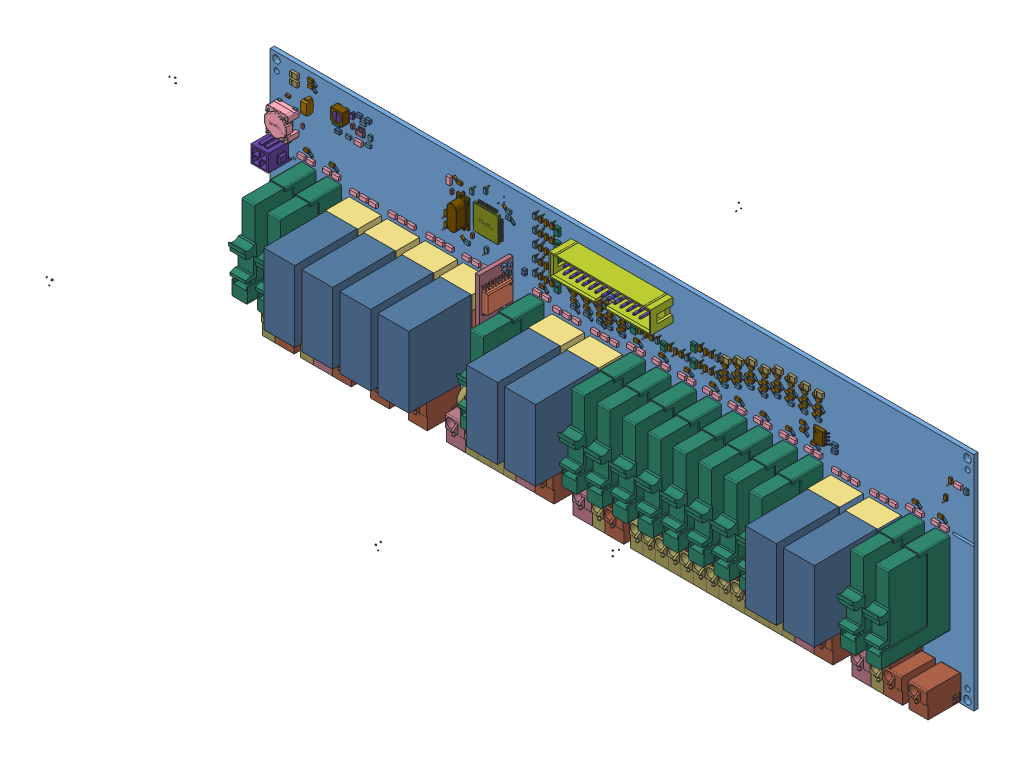
SolidWorks assembly _SC941C, configuration Default. Lengths in mm.
Overall size (350.55 148.76 148.76).
1847 component instances, 72 part files, 0 mates.
Components (placement in the parent):
- Board_1-1: Board_1 [Default] at (0 0 -1.6703) size (281.94 89 1.67)
- R93-1: R93 [Default] at origin size (0.8 1.6 0.55)
  - RESC1608X84N_1-1: RESC1608X84N_1 [Default] at (7.62 60.1979 0) x (0 -1 0) z (-1 0 0) size (1.6 0.55 0.8)
- R94-1: R94 [Default] at origin size (0.8 1.6 0.55)
  - RESC1608X84N_1-1: RESC1608X84N_1 [Default] at (-4.1442 60.201 0) x (0 -1 0) z (-1 0 0) size (1.6 0.55 0.8)
- L3-1: L3 [Default] at origin size (8.76 10 6)
  - STEP-744272102-rev1_RGB8421504-1: STEP-744272102-rev1_RGB8421504 [Default] at (1.7783 60.1986 0.3127) x (-1 0 0) z (0 0 1) size (8.76 10 6)
    - Base_1-1: Base_1 [Default] at origin size (5 6.5 2.6)
    - Base_2-1: Base_2 [Default] at origin size (8.76 10 5.3)
    - Base-1: Base [Default] at origin size (3.01 7.71 4.33)
    - Contact-1: Contact [Default] at (-3.11 -3.66 -0.3) x (-1 0 0) z (0 0 -1) size (1.2 1.83 6)
    - Contact-2: Contact [Default] at (3.11 -3.66 -0.3) x (-1 0 0) z (0 0 -1) size (1.2 1.83 6)
    - Contact-3: Contact [Default] at (-3.11 3.66 -0.3) x (1 0 0) z (0 0 -1) size (1.2 1.83 6)
    - Contact-4: Contact [Default] at (3.11 3.66 -0.3) x (1 0 0) z (0 0 -1) size (1.2 1.83 6)
- J3-1: J3 [Default] at origin size (40.68 9.1 12.1)
  - STEP-61202621621-rev1-1: STEP-61202621621-rev1 [Default] at (135.2551 70.2531 4.4377) x (1 0 0) z (0 0 1) size (40.68 9.1 12.1)
    - 61202621621-1: 61202621621 [Default] at origin size (40.68 9.1 9.1)
    - 6120xx21621_PIN-1: 6120xx21621_PIN [Default] at (-15.24 1.27 -1.875) size (0.64 0.64 11.6)
    - 6120xx21621_PIN-2: 6120xx21621_PIN [Default] at (-15.24 -1.27 -1.875) size (0.64 0.64 11.6)
    - 6120xx21621_PIN-3: 6120xx21621_PIN [Default] at (-12.7 1.27 -1.875) size (0.64 0.64 11.6)
    - 6120xx21621_PIN-4: 6120xx21621_PIN [Default] at (-10.16 1.27 -1.875) size (0.64 0.64 11.6)
    - 6120xx21621_PIN-5: 6120xx21621_PIN [Default] at (-12.7 -1.27 -1.875) size (0.64 0.64 11.6)
    - 6120xx21621_PIN-6: 6120xx21621_PIN [Default] at (-10.16 -1.27 -1.875) size (0.64 0.64 11.6)
    - 6120xx21621_PIN-7: 6120xx21621_PIN [Default] at (-7.62 1.27 -1.875) size (0.64 0.64 11.6)
    - 6120xx21621_PIN-8: 6120xx21621_PIN [Default] at (-7.62 -1.27 -1.875) size (0.64 0.64 11.6)
    - 6120xx21621_PIN-9: 6120xx21621_PIN [Default] at (-5.08 1.27 -1.875) size (0.64 0.64 11.6)
    - 6120xx21621_PIN-10: 6120xx21621_PIN [Default] at (-5.08 -1.27 -1.875) size (0.64 0.64 11.6)
    - 6120xx21621_PIN-11: 6120xx21621_PIN [Default] at (-2.54 1.27 -1.875) size (0.64 0.64 11.6)
    - 6120xx21621_PIN-12: 6120xx21621_PIN [Default] at (0 1.27 -1.875) size (0.64 0.64 11.6)
    - 6120xx21621_PIN-13: 6120xx21621_PIN [Default] at (-2.54 -1.27 -1.875) size (0.64 0.64 11.6)
    - 6120xx21621_PIN-14: 6120xx21621_PIN [Default] at (0 -1.27 -1.875) size (0.64 0.64 11.6)
    - 6120xx21621_PIN-15: 6120xx21621_PIN [Default] at (2.54 1.27 -1.875) size (0.64 0.64 11.6)
    - 6120xx21621_PIN-16: 6120xx21621_PIN [Default] at (2.54 -1.27 -1.875) size (0.64 0.64 11.6)
    - 6120xx21621_PIN-17: 6120xx21621_PIN [Default] at (5.08 1.27 -1.875) size (0.64 0.64 11.6)
    - 6120xx21621_PIN-18: 6120xx21621_PIN [Default] at (7.62 1.27 -1.875) size (0.64 0.64 11.6)
    - 6120xx21621_PIN-19: 6120xx21621_PIN [Default] at (5.08 -1.27 -1.875) size (0.64 0.64 11.6)
    - 6120xx21621_PIN-20: 6120xx21621_PIN [Default] at (7.62 -1.27 -1.875) size (0.64 0.64 11.6)
    - 6120xx21621_PIN-21: 6120xx21621_PIN [Default] at (10.16 1.27 -1.875) size (0.64 0.64 11.6)
    - 6120xx21621_PIN-22: 6120xx21621_PIN [Default] at (12.7 1.27 -1.875) size (0.64 0.64 11.6)
    - 6120xx21621_PIN-23: 6120xx21621_PIN [Default] at (10.16 -1.27 -1.875) size (0.64 0.64 11.6)
    - 6120xx21621_PIN-24: 6120xx21621_PIN [Default] at (12.7 -1.27 -1.875) size (0.64 0.64 11.6)
    - 6120xx21621_PIN-25: 6120xx21621_PIN [Default] at (15.24 1.27 -1.875) size (0.64 0.64 11.6)
    - 6120xx21621_PIN-26: 6120xx21621_PIN [Default] at (15.24 -1.27 -1.875) size (0.64 0.64 11.6)
- R45-1: R45 [Default] at origin size (3.3 1.97 0.78)
  - SW3dPS-0805_SMD_Resistor-1: SW3dPS-0805_SMD_Resistor [Default] at (141.4462 52.7049 0) x (-1 0 0) z (0 1 0) size (2 0.78 1.25)
  - 905261096-1: 905261096 [Default] at (143.2322 52.0303 0) size (1.03 1.35 0.76)
    - Extruded_2-1: Extruded_2 [Default] at origin size (1.03 1.35 0.76)
  - 905275240-1: 905275240 [Default] at (142.9941 52.1097 0) size (1.51 1.51 0.76)
    - Extruded_3-1: Extruded_3 [Default] at origin size (1.51 1.51 0.76)
  - 905265720-1: 905265720 [Default] at (143.1131 52.07 0) size (1.11 1.43 0.76)
    - Extruded_4-1: Extruded_4 [Default] at origin size (1.11 1.43 0.76)
- U1-1: U1 [Default] at origin size (3 3 1.35)
  - User_Library-SOT23-6-1: User_Library-SOT23-6 [Default] at (31.1467 69.8501 0) x (0 1 0) z (0 0 1) size (3 3 1.35)
- R2-1: R2 [Default] at origin size (1.2 2 0.7)
  - RESC2012X70N_1-1: RESC2012X70N_1 [Default] at (34.7981 69.6912 0) x (0 -1 0) z (-1 0 0) size (2 0.7 1.2)
- R4-1: R4 [Default] at origin size (2 1.2 0.7)
  - RESC2012X70N_1-1: RESC2012X70N_1 [Default] at (34.0042 66.6749 0) x (-1 0 0) z (0 1 0) size (2 0.7 1.2)
- R5-1: R5 [Default] at origin size (2 1.2 0.7)
  - RESC2012X70N_1-1: RESC2012X70N_1 [Default] at (31.9404 73.3424 0) x (-1 0 0) z (0 1 0) size (2 0.7 1.2)
- L2-1: L2 [Default] at origin size (3.2 1.6 1)
  - SW3dPS-1206_SMD_Resistor-1: SW3dPS-1206_SMD_Resistor [Default] at (21.463 68.2625 0) x (-1 0 0) z (0 1 0) size (3.2 1 1.6)
- L1-1: L1 [Default] at origin size (4.8 4.8 2.8)
  - WE-TPC_4828-1: WE-TPC_4828 [Default] at (23.6855 72.7074 2.794) x (-1 0 0) z (0 0 1) size (4.8 4.8 2.8)
    - base_3-1: base_3 [Default] at origin size (2.96 2.96 2.41)
    - base_4-1: base_4 [Default] at origin size (3.46 3.46 2.62)
    - base_5-1: base_5 [Default] at origin size (4.8 4.8 2.5)
    - base_6-1: base_6 [Default] at origin size (2.76 2.76 2.41)
    - Lötstreifen-1: Lötstreifen [Default] at (0 0 -2.8) x (-1 0 0) z (0 0 -1) size (1.6 4.8 0.3)
    - Lötstreifen_1-1: Lötstreifen_1 [Default] at (0 0 -2.8) x (-1 0 0) z (0 0 -1) size (1.6 4.8 0.3)
- D4-1: D4 [Default] at origin size (45.58 45.81 23.48)
  - SW3dPS-transistor_SOT233_4-1: SW3dPS-transistor_SOT233_4 [Default] at (-42.1069 42.9394 -21.9) x (-1 0 0) z (0 1 0) size (2.9 1.1 1.6)
  - SW3dPS-transistor_SOT233_5-1: SW3dPS-transistor_SOT233_5 [Default] at (-0.0421 0.0429 -0.0219) x (-1 0 0) z (0 1 0) size (2.18 2.18 2.18)
  - SW3dPS-transistor_SOT233_6-1: SW3dPS-transistor_SOT233_6 [Default] at (0 0 0) x (-1 0 0) z (0 1 0) size (2.18 2.18 2.18)
  - SW3dPS-transistor_SOT233_7-1: SW3dPS-transistor_SOT233_7 [Default] x (-1 0 0) z (0 1 0) size (2.18 2.18 2.18)
- D6-1: D6 [Default] at origin size (1.36 2.6 1.13)
  - SW3dPS-SOD-323-1: SW3dPS-SOD-323 [Default] at (27.8129 73.9776 0) x (0 1 0) z (0 0 1) size (2.6 1.36 1.13)
- D3-1: D3 [Default] at origin size (2.6 5.25 2.98)
  - SW3dPS-DO-214BA-1: SW3dPS-DO-214BA [Default] at (10.541 69.0721 1.9) x (-1 0 0) z (0 0 1) size (2.6 5.25 2.98)
- C4-1: C4 [Default] at origin size (2 1.25 1)
  - User_Library-CAPC2013X10-1: User_Library-CAPC2013X10 [Default] at (22.0981 65.7225 0) x (1 0 0) z (0 0 1) size (2 1.25 1)
- C1-1: C1 [Default] at origin size (2 1.25 1)
  - User_Library-CAPC2013X10-1: User_Library-CAPC2013X10 [Default] at (30.5116 75.4062 0) x (-1 0 0) z (0 0 1) size (2 1.25 1)
- C2-1: C2 [Default] at origin size (2 1.25 1)
  - User_Library-CAPC2013X10-1: User_Library-CAPC2013X10 [Default] at (34.1311 75.4062 0) x (-1 0 0) z (0 0 1) size (2 1.25 1)
- C3-1: C3 [Default] at origin size (0.8 1.6 0.9)
  - User_Library-CAPC1608X09_1-1: User_Library-CAPC1608X09_1 [Default] at (27.8131 70.3617 0) x (0 -1 0) z (0 0 1) size (1.6 0.8 0.9)
- VR1-1: VR1 [Default] at origin size (3.59 9 34)
  - WE-VD_7_mm-1: WE-VD_7_mm [Default] at (83.1849 8.3979 9) x (0 -1 0) z (0 0 1) size (9 3.59 34)
- U2-1: U2 [Default] at origin size (27.38 148.76 148.76)
  - SC943-0C_20-12-2012-1: SC943-0C_20-12-2012 [Default] at (91.5496 28.0022 3.7281) x (0 1 0.000663) z (1 0 0) size (148.66 148.66 27.38)
    - Board-1: Board [Default] at (0 0 -1.6167) size (43.5 16.8 1.62)
    - R15-1: R15 [Default] at origin size (1.6 0.8 0.55)
      - RESC1608X84N-1: RESC1608X84N [Default] at (-0.0001 1.9049 0) x (-1 0 0) z (0 1 0) size (1.6 0.55 0.8)
    - R11-1: R11 [Default] at origin size (2 1.2 0.7)
      - RESC2012X70N-1: RESC2012X70N [Default] at (-3.6513 -0.4763 0) x (-1 0 0) z (0 1 0) size (2 0.7 1.2)
    - R7-1: R7 [Default] at origin size (2 1.2 0.7)
      - RESC2012X70N-1: RESC2012X70N [Default] at (-5.2388 1.5874 0) x (-1 0 0) z (0 1 0) size (2 0.7 1.2)
    - D3_1-1: D3_1 [Default] at origin size (2.6 5.2 2.43)
      - SW3dPS-DO-214AC_SMA-1: SW3dPS-DO-214AC_SMA [Default] at (-1.4287 0.3175 -2.9167) x (1 0 0) z (0 0 -1) size (2.6 5.2 2.43)
    - T4-1: T4 [Default] at origin size (6.54 9.94 2.42)
      - SW3dPS-DPAK-1-1: SW3dPS-DPAK-1 [Default] at (10.9238 2.2758 -2.8167) x (1 0 0) z (0 1 0) size (6.54 2.42 9.94)
    - T3-1: T3 [Default] at origin size (6.54 9.94 2.42)
      - SW3dPS-DPAK-1-1: SW3dPS-DPAK-1 [Default] at (-10.3487 2.2758 -2.8167) x (1 0 0) z (0 1 0) size (6.54 2.42 9.94)
    - D5-1: D5 [Default] at origin size (2.6 5.2 2.43)
      - SW3dPS-DO-214AC_SMA-1: SW3dPS-DO-214AC_SMA [Default] at (2.0638 0.3175 -2.9167) x (1 0 0) z (0 0 -1) size (2.6 5.2 2.43)
    - D4_1-1: D4_1 [Default] at origin size (2.6 5.2 2.43)
      - SW3dPS-DO-214AC_SMA-1: SW3dPS-DO-214AC_SMA [Default] at (5.2388 0.3175 -2.9167) x (1 0 0) z (0 0 -1) size (2.6 5.2 2.43)
    - D2-1: D2 [Default] at origin size (2.6 5.2 2.43)
      - SW3dPS-DO-214AC_SMA-1: SW3dPS-DO-214AC_SMA [Default] at (-4.6037 0.3175 -2.9167) x (1 0 0) z (0 0 -1) size (2.6 5.2 2.43)
    - R25-1: R25 [Default] at origin size (3.2 1.6 0.84)
      - RESC3216X84N-1: RESC3216X84N [Default] at (-2.0851 5.5563 -1.6167) x (-1 0 0) z (0 -1 0) size (3.2 0.84 1.6)
    - R26-1: R26 [Default] at origin size (3.2 1.6 0.84)
      - RESC3216X84N-1: RESC3216X84N [Default] at (2.6989 5.5562 -1.6167) x (1 0 0) z (0 1 0) size (3.2 0.84 1.6)
    - C6-1: C6 [Default] at origin size (0.8 1.6 0.9)
      - User_Library-CAPC1608X09-1: User_Library-CAPC1608X09 [Default] at (10.0013 0.1587 0) x (0 -1 0) z (0 0 1) size (1.6 0.8 0.9)
    - C7-1: C7 [Default] at origin size (0.8 1.6 0.9)
      - User_Library-CAPC1608X09-1: User_Library-CAPC1608X09 [Default] at (27.7813 0.1587 0) x (0 -1 0) z (0 0 1) size (1.6 0.8 0.9)
    - C8-1: C8 [Default] at origin size (0.8 1.6 0.9)
      - User_Library-CAPC1608X09-1: User_Library-CAPC1608X09 [Default] at (26.1938 0.1587 0) x (0 -1 0) z (0 0 1) size (1.6 0.8 0.9)
    - C9-1: C9 [Default] at origin size (1.6 0.8 0.9)
      - User_Library-CAPC1608X09-1: User_Library-CAPC1608X09 [Default] at (7.7788 2.3813 0) size (1.6 0.8 0.9)
    - L1_1-1: L1_1 [Default] at origin size (1.6 0.8 0.9)
      - User_Library-CAPC1608X09-1: User_Library-CAPC1608X09 [Default] at (10.7949 -2.0638 0) x (-1 0 0) z (0 0 1) size (1.6 0.8 0.9)
    - L2_1-1: L2_1 [Default] at origin size (1.6 0.8 0.9)
      - User_Library-CAPC1608X09-1: User_Library-CAPC1608X09 [Default] at (27.1463 -2.2224 0) size (1.6 0.8 0.9)
    - L3_1-1: L3_1 [Default] at origin size (1.6 0.8 0.9)
      - User_Library-CAPC1608X09-1: User_Library-CAPC1608X09 [Default] at (10.7949 2.3812 0) x (-1 0 0) z (0 0 1) size (1.6 0.8 0.9)
    - U1_1-1: U1_1 [Default] at origin size (10.3 10.3 2.65)
      - SW3dPS-SOIC16-300-1: SW3dPS-SOIC16-300 [Default] at (19.685 3.9689 0) x (0 1 0) z (0 0 1) size (10.3 10.3 2.65)
    - R2_1-1: R2_1 [Default] at origin size (2 1.2 0.7)
      - RESC2012X70N-1: RESC2012X70N [Default] at (-8.7312 1.9051 0) x (1 0 0) z (0 -1 0) size (2 0.7 1.2)
    - C4_1-1: C4_1 [Default] at origin size (0.8 1.6 0.9)
      - User_Library-CAPC1608X09-1: User_Library-CAPC1608X09 [Default] at (-13.0176 7.6201 0) x (0 1 0) z (0 0 1) size (1.6 0.8 0.9)
    - T6-1: T6 [Default] at origin size (36.29 81.18 23.48)
      - SW3dPS-transistor_SOT233-1: SW3dPS-transistor_SOT233 [Default] at (-33.4193 77.6987 -21.9) x (0 1 0) z (1 0 0) size (2.9 1.1 1.6)
      - SW3dPS-transistor_SOT233_1-1: SW3dPS-transistor_SOT233_1 [Default] at (-0.0334 0.0777 -0.0219) x (0 1 0) z (1 0 0) size (2.18 2.18 2.18)
      - SW3dPS-transistor_SOT233_2-1: SW3dPS-transistor_SOT233_2 [Default] at (0 0.0001 0) x (0 1 0) z (1 0 0) size (2.18 2.18 2.18)
      - SW3dPS-transistor_SOT233_3-1: SW3dPS-transistor_SOT233_3 [Default] x (0 1 0) z (1 0 0) size (2.18 2.18 2.18)
    - U2_1-1: U2_1 [Default] at origin size (6.2 5 1.75)
      - User_Library-SOIC-8-150-1: User_Library-SOIC-8-150 [Default] at (6.9849 6.3501 1) x (0 -1 0) z (-1 0 0) size (5 1.75 6.2)
        - User_Library-SOIC-8-150_pin_SOIC_SO-150_1_1-1: User_Library-SOIC-8-150_pin_SOIC_SO-150_1_1 [Default] at (0.6 0 -2) x (-1 0 0) z (0 0 -1) size (0.4 1.1 1.1)
        - User_Library-SOIC-8-150_pin_SOIC_SO-150_1_1-2: User_Library-SOIC-8-150_pin_SOIC_SO-150_1_1 [Default] at (-0.67 0 -2) x (-1 0 0) z (0 0 -1) size (0.4 1.1 1.1)
        - User_Library-SOIC-8-150_pin_SOIC_SO-150_1_1-3: User_Library-SOIC-8-150_pin_SOIC_SO-150_1_1 [Default] at (-1.94 0 2) size (0.4 1.1 1.1)
        - User_Library-SOIC-8-150_pin_SOIC_SO-150_1_1-4: User_Library-SOIC-8-150_pin_SOIC_SO-150_1_1 [Default] at (-0.67 0 2) size (0.4 1.1 1.1)
        - User_Library-SOIC-8-150_pin_SOIC_SO-150_1_1-5: User_Library-SOIC-8-150_pin_SOIC_SO-150_1_1 [Default] at (-1.94 0 -2) x (-1 0 0) z (0 0 -1) size (0.4 1.1 1.1)
        - User_Library-SOIC-8-150_pin_SOIC_SO-150_1_1-6: User_Library-SOIC-8-150_pin_SOIC_SO-150_1_1 [Default] at (1.87 0 2) size (0.4 1.1 1.1)
        - User_Library-SOIC-8-150_SOIC_150_SOIC_5X4_1_1-1: User_Library-SOIC-8-150_SOIC_150_SOIC_5X4_1_1 [Default] at origin size (5 1.5 4)
        - User_Library-SOIC-8-150_pin_SOIC_SO-150_1_1-7: User_Library-SOIC-8-150_pin_SOIC_SO-150_1_1 [Default] at (0.6 0 2) size (0.4 1.1 1.1)
        - User_Library-SOIC-8-150_pin_SOIC_SO-150_1_1-8: User_Library-SOIC-8-150_pin_SOIC_SO-150_1_1 [Default] at (1.87 0 -2) x (-1 0 0) z (0 0 -1) size (0.4 1.1 1.1)
    - R16-1: R16 [Default] at origin size (1.2 2 0.7)
      - RESC2012X70N-1: RESC2012X70N [Default] at (-3.1751 7.3026 0) x (0 1 0) z (1 0 0) size (2 0.7 1.2)
    - R12-1: R12 [Default] at origin size (1.2 2 0.7)
      - RESC2012X70N-1: RESC2012X70N [Default] at (2.2226 -1.2701 0) x (0 -1 0) z (-1 0 0) size (2 0.7 1.2)
    - R9-1: R9 [Default] at origin size (1.6 0.8 0.55)
      - RESC1608X84N-1: RESC1608X84N [Default] at (1.5874 5.5562 0) x (-1 0 0) z (0 1 0) size (1.6 0.55 0.8)
    - R8-1: R8 [Default] at origin size (2 1.2 0.7)
      - RESC2012X70N-1: RESC2012X70N [Default] at (5.0801 -1.9049 0) x (1 0 0) z (0 -1 0) size (2 0.7 1.2)
    - C5-1: C5 [Default] at origin size (0.8 1.6 0.9)
      - User_Library-CAPC1608X09-1: User_Library-CAPC1608X09 [Default] at (11.5888 0.1587 0) x (0 -1 0) z (0 0 1) size (1.6 0.8 0.9)
    - C3_1-1: C3_1 [Default] at origin size (0.8 1.6 0.9)
      - User_Library-CAPC1608X09-1: User_Library-CAPC1608X09 [Default] at (8.4138 0.1587 0) x (0 -1 0) z (0 0 1) size (1.6 0.8 0.9)
    - C2_1-1: C2_1 [Default] at origin size (0.8 1.6 0.9)
      - User_Library-CAPC1608X09-1: User_Library-CAPC1608X09 [Default] at (13.1763 0.1587 0) x (0 -1 0) z (0 0 1) size (1.6 0.8 0.9)
    - R17-1: R17 [Default] at origin size (0.8 1.6 0.55)
      - RESC1608X84N-1: RESC1608X84N [Default] at (-1.2701 7.6201 0) x (0 1 0) z (1 0 0) size (1.6 0.55 0.8)
    - R18-1: R18 [Default] at origin size (1.6 0.8 0.55)
      - RESC1608X84N-1: RESC1608X84N [Default] at (-6.9851 8.2549 0) x (-1 0 0) z (0 1 0) size (1.6 0.55 0.8)
    - T5-1: T5 [Default] at origin size (82.76 20.1 23.48)
      - SW3dPS-transistor_SOT233-1: SW3dPS-transistor_SOT233 [Default] at (-79.2862 -17.2268 -21.9) x (-1 0 0) z (0 1 0) size (2.9 1.1 1.6)
      - SW3dPS-transistor_SOT233_1-1: SW3dPS-transistor_SOT233_1 [Default] at (-0.0793 -0.0172 -0.0219) x (-1 0 0) z (0 1 0) size (2.18 2.18 2.18)
      - SW3dPS-transistor_SOT233_2-1: SW3dPS-transistor_SOT233_2 [Default] at (-0.0001 0 0) x (-1 0 0) z (0 1 0) size (2.18 2.18 2.18)
      - SW3dPS-transistor_SOT233_3-1: SW3dPS-transistor_SOT233_3 [Default] x (-1 0 0) z (0 1 0) size (2.18 2.18 2.18)
    - T7-1: T7 [Default] at origin size (73.54 29.78 23.48)
      - SW3dPS-transistor_SOT233-1: SW3dPS-transistor_SOT233 [Default] at (70.0609 26.9106 -21.9) x (1 0 0) z (0 -1 0) size (2.9 1.1 1.6)
      - SW3dPS-transistor_SOT233_1-1: SW3dPS-transistor_SOT233_1 [Default] at (0.0701 0.0269 -0.0219) x (1 0 0) z (0 -1 0) size (2.18 2.18 2.18)
      - SW3dPS-transistor_SOT233_2-1: SW3dPS-transistor_SOT233_2 [Default] at (0.0001 0 0) x (1 0 0) z (0 -1 0) size (2.18 2.18 2.18)
      - SW3dPS-transistor_SOT233_3-1: SW3dPS-transistor_SOT233_3 [Default] x (1 0 0) z (0 -1 0) size (2.18 2.18 2.18)
    - C1_1-1: C1_1 [Default] at origin size (1.6 0.8 0.9)
      - User_Library-CAPC1608X09-1: User_Library-CAPC1608X09 [Default] at (27.1462 -1.9049 -1.6167) x (-1 0 0) z (0 0 -1) size (1.6 0.8 0.9)
    - R19-1: R19 [Default] at origin size (1.6 0.8 0.55)
      - RESC1608X84N-1: RESC1608X84N [Default] at (-10.7949 8.2551 0) x (1 0 0) z (0 -1 0) size (1.6 0.55 0.8)
    - R1-1: R1 [Default] at origin size (1.6 0.8 0.55)
      - RESC1608X84N-1: RESC1608X84N [Default] at (24.1301 -2.2224 0) x (1 0 0) z (0 -1 0) size (1.6 0.55 0.8)
    - D1-1: D1 [Default] at origin size (80.06 27.08 23.48)
      - SW3dPS-transistor_SOT233-1: SW3dPS-transistor_SOT233 [Default] at (76.5874 24.2118 -21.9) x (1 0 0) z (0 -1 0) size (2.9 1.1 1.6)
      - SW3dPS-transistor_SOT233_1-1: SW3dPS-transistor_SOT233_1 [Default] at (0.0766 0.0242 -0.0219) x (1 0 0) z (0 -1 0) size (2.18 2.18 2.18)
      - SW3dPS-transistor_SOT233_2-1: SW3dPS-transistor_SOT233_2 [Default] at (0.0001 0 0) x (1 0 0) z (0 -1 0) size (2.18 2.18 2.18)
      - SW3dPS-transistor_SOT233_3-1: SW3dPS-transistor_SOT233_3 [Default] x (1 0 0) z (0 -1 0) size (2.18 2.18 2.18)
    - D6_1-1: D6_1 [Default] at origin size (13.75 77.05 23.48)
      - SW3dPS-transistor_SOT233-1: SW3dPS-transistor_SOT233 [Default] at (10.8768 -73.5712 -21.9) x (0 -1 0) z (-1 0 0) size (2.9 1.1 1.6)
      - SW3dPS-transistor_SOT233_1-1: SW3dPS-transistor_SOT233_1 [Default] at (0.0109 -0.0736 -0.0219) x (0 -1 0) z (-1 0 0) size (2.18 2.18 2.18)
      - SW3dPS-transistor_SOT233_2-1: SW3dPS-transistor_SOT233_2 [Default] at (0 -0.0001 0) x (0 -1 0) z (-1 0 0) size (2.18 2.18 2.18)
      - SW3dPS-transistor_SOT233_3-1: SW3dPS-transistor_SOT233_3 [Default] x (0 -1 0) z (-1 0 0) size (2.18 2.18 2.18)
    - D7-1: D7 [Default] at origin size (17.72 77.05 23.48)
      - SW3dPS-transistor_SOT233-1: SW3dPS-transistor_SOT233 [Default] at (14.8456 -73.5712 -21.9) x (0 -1 0) z (-1 0 0) size (2.9 1.1 1.6)
      - SW3dPS-transistor_SOT233_1-1: SW3dPS-transistor_SOT233_1 [Default] at (0.0148 -0.0736 -0.0219) x (0 -1 0) z (-1 0 0) size (2.18 2.18 2.18)
      - SW3dPS-transistor_SOT233_2-1: SW3dPS-transistor_SOT233_2 [Default] at (0 -0.0001 0) x (0 -1 0) z (-1 0 0) size (2.18 2.18 2.18)
      - SW3dPS-transistor_SOT233_3-1: SW3dPS-transistor_SOT233_3 [Default] x (0 -1 0) z (-1 0 0) size (2.18 2.18 2.18)
    - R3-1: R3 [Default] at origin size (2 1.2 0.7)
      - RESC2012X70N-1: RESC2012X70N [Default] at (-12.2237 1.9051 0) x (1 0 0) z (0 -1 0) size (2 0.7 1.2)
- C15-1: C15 [Default] at origin size (1.25 2 1)
  - User_Library-CAPC2013X10-1: User_Library-CAPC2013X10 [Default] at (96.6787 54.2924 0) x (0 -1 0) z (0 0 1) size (2 1.25 1)
- R22-1: R22 [Default] at origin size (3.3 1.97 0.78)
  - SW3dPS-0805_SMD_Resistor-1: SW3dPS-0805_SMD_Resistor [Default] at (116.2051 56.5151 0) x (1 0 0) z (0 -1 0) size (2 0.78 1.25)
  - 905266264-1: 905266264 [Default] at (114.4191 57.1897 0) size (1.03 1.35 0.76)
    - Extruded_14-1: Extruded_14 [Default] at origin size (1.03 1.35 0.76)
  - 905263816-1: 905263816 [Default] at (114.6572 57.1103 0) size (1.51 1.51 0.76)
    - Extruded_15-1: Extruded_15 [Default] at origin size (1.51 1.51 0.76)
  - 905266536-1: 905266536 [Default] at (114.5381 57.15 0) size (1.11 1.43 0.76)
    - Extruded_16-1: Extruded_16 [Default] at origin size (1.11 1.43 0.76)
- R20-1: R20 [Default] at origin size (3.3 1.97 0.78)
  - SW3dPS-0805_SMD_Resistor-1: SW3dPS-0805_SMD_Resistor [Default] at (116.2049 58.8009 0) x (-1 0 0) z (0 1 0) size (2 0.78 1.25)
  - 905261096-1: 905261096 [Default] at (117.9909 58.1263 0) size (1.03 1.35 0.76)
    - Extruded_2-1: Extruded_2 [Default] at origin size (1.03 1.35 0.76)
  - 905275240-1: 905275240 [Default] at (117.7528 58.2057 0) size (1.51 1.51 0.76)
    - Extruded_3-1: Extruded_3 [Default] at origin size (1.51 1.51 0.76)
  - 905265720-1: 905265720 [Default] at (117.8719 58.166 0) size (1.11 1.43 0.76)
    - Extruded_4-1: Extruded_4 [Default] at origin size (1.11 1.43 0.76)
- D15-1: D15 [Default] at origin size (2.9 1.9 0.99)
  - 905269392-1: 905269392 [Default] at (115.697 61.087 0) size (2.9 1.9 0.98)
    - Extruded_17-1: Extruded_17 [Default] at origin size (2.9 1.9 0.98)
  - 905269800-1: 905269800 [Default] at (116.332 61.087 0.95) size (0.25 1.78 0.04)
    - Extruded_18-1: Extruded_18 [Default] at origin size (0.25 1.78 0.04)
- C9_1-1: C9_1 [Default] at origin size (3.3 1.97 0.78)
  - SW3dPS-0805_SMD_Capacitor-1: SW3dPS-0805_SMD_Capacitor [Default] at (116.2049 51.943 0) x (-1 0 0) z (0 1 0) size (2 0.78 1.25)
  - 905265720-1: 905265720 [Default] at (117.8719 51.308 0) size (1.11 1.43 0.76)
    - Extruded_4-1: Extruded_4 [Default] at origin size (1.11 1.43 0.76)
  - 905275240-1: 905275240 [Default] at (117.7528 51.3477 0) size (1.51 1.51 0.76)
    - Extruded_3-1: Extruded_3 [Default] at origin size (1.51 1.51 0.76)
  - 905261096-1: 905261096 [Default] at (117.9909 51.2683 0) size (1.03 1.35 0.76)
    - Extruded_2-1: Extruded_2 [Default] at origin size (1.03 1.35 0.76)
- T29-1: T29 [Default] at origin size (337.24 75.5 23.48)
  - SW3dPS-transistor_SOT233_4-1: SW3dPS-transistor_SOT233_4 [Default] at (333.7624 72.6306 -21.9) x (1 0 0) z (0 -1 0) size (2.9 1.1 1.6)
  - SW3dPS-transistor_SOT233_5-1: SW3dPS-transistor_SOT233_5 [Default] at (0.3338 0.0726 -0.0219) x (1 0 0) z (0 -1 0) size (2.18 2.18 2.18)
  - SW3dPS-transistor_SOT233_6-1: SW3dPS-transistor_SOT233_6 [Default] at (0.0003 0.0001 0) x (1 0 0) z (0 -1 0) size (2.18 2.18 2.18)
  - SW3dPS-transistor_SOT233_7-1: SW3dPS-transistor_SOT233_7 [Default] x (1 0 0) z (0 -1 0) size (2.18 2.18 2.18)
- T28-1: T28 [Default] at origin size (327.08 75.5 23.48)
  - SW3dPS-transistor_SOT233_4-1: SW3dPS-transistor_SOT233_4 [Default] at (323.6024 72.6306 -21.9) x (1 0 0) z (0 -1 0) size (2.9 1.1 1.6)
  - SW3dPS-transistor_SOT233_5-1: SW3dPS-transistor_SOT233_5 [Default] at (0.3236 0.0726 -0.0219) x (1 0 0) z (0 -1 0) size (2.18 2.18 2.18)
  - SW3dPS-transistor_SOT233_6-1: SW3dPS-transistor_SOT233_6 [Default] at (0.0003 0.0001 0) x (1 0 0) z (0 -1 0) size (2.18 2.18 2.18)
  - SW3dPS-transistor_SOT233_7-1: SW3dPS-transistor_SOT233_7 [Default] x (1 0 0) z (0 -1 0) size (2.18 2.18 2.18)
- T11-1: T11 [Default] at origin size (177.54 75.5 23.48)
  - SW3dPS-transistor_SOT233_4-1: SW3dPS-transistor_SOT233_4 [Default] at (174.0599 72.6306 -21.9) x (1 0 0) z (0 -1 0) size (2.9 1.1 1.6)
  - SW3dPS-transistor_SOT233_5-1: SW3dPS-transistor_SOT233_5 [Default] at (0.1741 0.0726 -0.0219) x (1 0 0) z (0 -1 0) size (2.18 2.18 2.18)
  - SW3dPS-transistor_SOT233_6-1: SW3dPS-transistor_SOT233_6 [Default] at (0.0002 0.0001 0) x (1 0 0) z (0 -1 0) size (2.18 2.18 2.18)
  - SW3dPS-transistor_SOT233_7-1: SW3dPS-transistor_SOT233_7 [Default] x (1 0 0) z (0 -1 0) size (2.18 2.18 2.18)
- T22-1: T22 [Default] at origin size (276.28 75.5 23.48)
  - SW3dPS-transistor_SOT233_4-1: SW3dPS-transistor_SOT233_4 [Default] at (272.8024 72.6306 -21.9) x (1 0 0) z (0 -1 0) size (2.9 1.1 1.6)
  - SW3dPS-transistor_SOT233_5-1: SW3dPS-transistor_SOT233_5 [Default] at (0.2728 0.0726 -0.0219) x (1 0 0) z (0 -1 0) size (2.18 2.18 2.18)
  - SW3dPS-transistor_SOT233_6-1: SW3dPS-transistor_SOT233_6 [Default] at (0.0003 0.0001 0) x (1 0 0) z (0 -1 0) size (2.18 2.18 2.18)
  - SW3dPS-transistor_SOT233_7-1: SW3dPS-transistor_SOT233_7 [Default] x (1 0 0) z (0 -1 0) size (2.18 2.18 2.18)
- T2-1: T2 [Default] at origin size (93.4 75.5 23.48)
  - SW3dPS-transistor_SOT233_4-1: SW3dPS-transistor_SOT233_4 [Default] at (89.9224 72.6306 -21.9) x (1 0 0) z (0 -1 0) size (2.9 1.1 1.6)
  - SW3dPS-transistor_SOT233_5-1: SW3dPS-transistor_SOT233_5 [Default] at (0.0899 0.0726 -0.0219) x (1 0 0) z (0 -1 0) size (2.18 2.18 2.18)
  - SW3dPS-transistor_SOT233_6-1: SW3dPS-transistor_SOT233_6 [Default] at (0.0001 0.0001 0) x (1 0 0) z (0 -1 0) size (2.18 2.18 2.18)
  - SW3dPS-transistor_SOT233_7-1: SW3dPS-transistor_SOT233_7 [Default] x (1 0 0) z (0 -1 0) size (2.18 2.18 2.18)
- T1-1: T1 [Default] at origin size (83.24 75.5 23.48)
  - SW3dPS-transistor_SOT233_4-1: SW3dPS-transistor_SOT233_4 [Default] at (79.7624 72.6306 -21.9) x (1 0 0) z (0 -1 0) size (2.9 1.1 1.6)
  - SW3dPS-transistor_SOT233_5-1: SW3dPS-transistor_SOT233_5 [Default] at (0.0798 0.0726 -0.0219) x (1 0 0) z (0 -1 0) size (2.18 2.18 2.18)
  - SW3dPS-transistor_SOT233_6-1: SW3dPS-transistor_SOT233_6 [Default] at (0.0001 0.0001 0) x (1 0 0) z (0 -1 0) size (2.18 2.18 2.18)
  - SW3dPS-transistor_SOT233_7-1: SW3dPS-transistor_SOT233_7 [Default] x (1 0 0) z (0 -1 0) size (2.18 2.18 2.18)
- R89-1: R89 [Default] at origin size (3.3 1.97 0.78)
  - SW3dPS-0805_SMD_Resistor-1: SW3dPS-0805_SMD_Resistor [Default] at (263.3662 52.7049 0) x (-1 0 0) z (0 1 0) size (2 0.78 1.25)
  - 905261096-1: 905261096 [Default] at (265.1522 52.0303 0) size (1.03 1.35 0.76)
    - Extruded_2-1: Extruded_2 [Default] at origin size (1.03 1.35 0.76)
  - 905275240-1: 905275240 [Default] at (264.9141 52.1097 0) size (1.51 1.51 0.76)
    - Extruded_3-1: Extruded_3 [Default] at origin size (1.51 1.51 0.76)
  - 905265720-1: 905265720 [Default] at (265.0331 52.07 0) size (1.11 1.43 0.76)
    - Extruded_4-1: Extruded_4 [Default] at origin size (1.11 1.43 0.76)
- R72-1: R72 [Default] at origin size (3.3 1.97 0.78)
  - SW3dPS-0805_SMD_Resistor-1: SW3dPS-0805_SMD_Resistor [Default] at (212.5662 52.7049 0) x (-1 0 0) z (0 1 0) size (2 0.78 1.25)
  - 905261096-1: 905261096 [Default] at (214.3522 52.0303 0) size (1.03 1.35 0.76)
    - Extruded_2-1: Extruded_2 [Default] at origin size (1.03 1.35 0.76)
  - 905275240-1: 905275240 [Default] at (214.1141 52.1097 0) size (1.51 1.51 0.76)
    - Extruded_3-1: Extruded_3 [Default] at origin size (1.51 1.51 0.76)
  - 905265720-1: 905265720 [Default] at (214.2331 52.07 0) size (1.11 1.43 0.76)
    - Extruded_4-1: Extruded_4 [Default] at origin size (1.11 1.43 0.76)
- R7_1-1: R7_1 [Default] at origin size (3.3 1.97 0.78)
  - SW3dPS-0805_SMD_Resistor-1: SW3dPS-0805_SMD_Resistor [Default] at (19.5262 52.7049 0) x (-1 0 0) z (0 1 0) size (2 0.78 1.25)
  - 905261096-1: 905261096 [Default] at (21.3122 52.0303 0) size (1.03 1.35 0.76)
    - Extruded_2-1: Extruded_2 [Default] at origin size (1.03 1.35 0.76)
  - 905275240-1: 905275240 [Default] at (21.0741 52.1097 0) size (1.51 1.51 0.76)
    - Extruded_3-1: Extruded_3 [Default] at origin size (1.51 1.51 0.76)
  - 905265720-1: 905265720 [Default] at (21.1931 52.07 0) size (1.11 1.43 0.76)
    - Extruded_4-1: Extruded_4 [Default] at origin size (1.11 1.43 0.76)
- R60-1: R60 [Default] at origin size (3.3 1.97 0.78)
  - SW3dPS-0805_SMD_Resistor-1: SW3dPS-0805_SMD_Resistor [Default] at (182.0862 52.7049 0) x (-1 0 0) z (0 1 0) size (2 0.78 1.25)
  - 905261096-1: 905261096 [Default] at (183.8722 52.0303 0) size (1.03 1.35 0.76)
    - Extruded_2-1: Extruded_2 [Default] at origin size (1.03 1.35 0.76)
  - 905275240-1: 905275240 [Default] at (183.6341 52.1097 0) size (1.51 1.51 0.76)
    - Extruded_3-1: Extruded_3 [Default] at origin size (1.51 1.51 0.76)
  - 905265720-1: 905265720 [Default] at (183.7531 52.07 0) size (1.11 1.43 0.76)
    - Extruded_4-1: Extruded_4 [Default] at origin size (1.11 1.43 0.76)
- K11-1: K11 [Default] at origin size (6.2 33 32.7)
  - User_Library-93_11-1: User_Library-93_11 [Default] at (148.665 47.3038 0) x (0 -1 0) z (0 0 1) size (33 6.2 32.7)
- K10-1: K10 [Default] at origin size (6.2 33 32.7)
  - User_Library-93_11-1: User_Library-93_11 [Default] at (138.505 47.3038 0) x (0 -1 0) z (0 0 1) size (33 6.2 32.7)
- K17-1: K17 [Default] at origin size (6.2 33 32.7)
  - User_Library-93_11-1: User_Library-93_11 [Default] at (209.625 47.3038 0) x (0 -1 0) z (0 0 1) size (33 6.2 32.7)
- K1-1: K1 [Default] at origin size (6.2 33 32.7)
  - User_Library-93_11-1: User_Library-93_11 [Default] at (6.425 47.3038 0) x (0 -1 0) z (0 0 1) size (33 6.2 32.7)
- D49-1: D49 [Default] at origin size (196.12 29.62 23.48)
  - SW3dPS-transistor_SOT233_4-1: SW3dPS-transistor_SOT233_4 [Default] at (192.8113 26.7469 -21.9) x (-1 0 0) z (0 1 0) size (2.9 1.1 1.6)
  - SW3dPS-transistor_SOT233_5-1: SW3dPS-transistor_SOT233_5 [Default] at (0.1928 0.0267 -0.0219) x (-1 0 0) z (0 1 0) size (2.18 2.18 2.18)
  - SW3dPS-transistor_SOT233_6-1: SW3dPS-transistor_SOT233_6 [Default] at (0.0002 0 0) x (-1 0 0) z (0 1 0) size (2.18 2.18 2.18)
  - SW3dPS-transistor_SOT233_7-1: SW3dPS-transistor_SOT233_7 [Default] x (-1 0 0) z (0 1 0) size (2.18 2.18 2.18)
- D27-1: D27 [Default] at origin size (74.32 29.62 23.48)
  - SW3dPS-transistor_SOT233_4-1: SW3dPS-transistor_SOT233_4 [Default] at (70.8913 26.7469 -21.9) x (-1 0 0) z (0 1 0) size (2.9 1.1 1.6)
  - SW3dPS-transistor_SOT233_5-1: SW3dPS-transistor_SOT233_5 [Default] at (0.0709 0.0267 -0.0219) x (-1 0 0) z (0 1 0) size (2.18 2.18 2.18)
  - SW3dPS-transistor_SOT233_6-1: SW3dPS-transistor_SOT233_6 [Default] at (0.0001 0 0) x (-1 0 0) z (0 1 0) size (2.18 2.18 2.18)
  - SW3dPS-transistor_SOT233_7-1: SW3dPS-transistor_SOT233_7 [Default] x (-1 0 0) z (0 1 0) size (2.18 2.18 2.18)
- D38-1: D38 [Default] at origin size (135.22 29.62 23.48)
  - SW3dPS-transistor_SOT233_4-1: SW3dPS-transistor_SOT233_4 [Default] at (131.8513 26.7469 -21.9) x (-1 0 0) z (0 1 0) size (2.9 1.1 1.6)
  - SW3dPS-transistor_SOT233_5-1: SW3dPS-transistor_SOT233_5 [Default] at (0.1319 0.0267 -0.0219) x (-1 0 0) z (0 1 0) size (2.18 2.18 2.18)
  - SW3dPS-transistor_SOT233_6-1: SW3dPS-transistor_SOT233_6 [Default] at (0.0001 0 0) x (-1 0 0) z (0 1 0) size (2.18 2.18 2.18)
  - SW3dPS-transistor_SOT233_7-1: SW3dPS-transistor_SOT233_7 [Default] x (-1 0 0) z (0 1 0) size (2.18 2.18 2.18)
- D36-1: D36 [Default] at origin size (125.07 29.62 23.48)
  - SW3dPS-transistor_SOT233_4-1: SW3dPS-transistor_SOT233_4 [Default] at (121.6913 26.7469 -21.9) x (-1 0 0) z (0 1 0) size (2.9 1.1 1.6)
  - SW3dPS-transistor_SOT233_5-1: SW3dPS-transistor_SOT233_5 [Default] at (0.1217 0.0267 -0.0219) x (-1 0 0) z (0 1 0) size (2.18 2.18 2.18)
  - SW3dPS-transistor_SOT233_6-1: SW3dPS-transistor_SOT233_6 [Default] at (0.0001 0 0) x (-1 0 0) z (0 1 0) size (2.18 2.18 2.18)
  - SW3dPS-transistor_SOT233_7-1: SW3dPS-transistor_SOT233_7 [Default] x (-1 0 0) z (0 1 0) size (2.18 2.18 2.18)
- D34-1: D34 [Default] at origin size (114.92 29.62 23.48)
  - SW3dPS-transistor_SOT233_4-1: SW3dPS-transistor_SOT233_4 [Default] at (111.5313 26.7469 -21.9) x (-1 0 0) z (0 1 0) size (2.9 1.1 1.6)
  - SW3dPS-transistor_SOT233_5-1: SW3dPS-transistor_SOT233_5 [Default] at (0.1115 0.0267 -0.0219) x (-1 0 0) z (0 1 0) size (2.18 2.18 2.18)
  - SW3dPS-transistor_SOT233_6-1: SW3dPS-transistor_SOT233_6 [Default] at (0.0001 0 0) x (-1 0 0) z (0 1 0) size (2.18 2.18 2.18)
  - SW3dPS-transistor_SOT233_7-1: SW3dPS-transistor_SOT233_7 [Default] x (-1 0 0) z (0 1 0) size (2.18 2.18 2.18)
- T17-1: T17 [Default] at origin size (225.48 75.5 23.48)
  - SW3dPS-transistor_SOT233_4-1: SW3dPS-transistor_SOT233_4 [Default] at (222.0024 72.6306 -21.9) x (1 0 0) z (0 -1 0) size (2.9 1.1 1.6)
  - SW3dPS-transistor_SOT233_5-1: SW3dPS-transistor_SOT233_5 [Default] at (0.222 0.0726 -0.0219) x (1 0 0) z (0 -1 0) size (2.18 2.18 2.18)
  - SW3dPS-transistor_SOT233_6-1: SW3dPS-transistor_SOT233_6 [Default] at (0.0002 0.0001 0) x (1 0 0) z (0 -1 0) size (2.18 2.18 2.18)
  - SW3dPS-transistor_SOT233_7-1: SW3dPS-transistor_SOT233_7 [Default] x (1 0 0) z (0 -1 0) size (2.18 2.18 2.18)
- T23-1: T23 [Default] at origin size (286.44 75.5 23.48)
  - SW3dPS-transistor_SOT233_4-1: SW3dPS-transistor_SOT233_4 [Default] at (282.9624 72.6306 -21.9) x (1 0 0) z (0 -1 0) size (2.9 1.1 1.6)
  - SW3dPS-transistor_SOT233_5-1: SW3dPS-transistor_SOT233_5 [Default] at (0.283 0.0726 -0.0219) x (1 0 0) z (0 -1 0) size (2.18 2.18 2.18)
  - SW3dPS-transistor_SOT233_6-1: SW3dPS-transistor_SOT233_6 [Default] at (0.0003 0.0001 0) x (1 0 0) z (0 -1 0) size (2.18 2.18 2.18)
  - SW3dPS-transistor_SOT233_7-1: SW3dPS-transistor_SOT233_7 [Default] x (1 0 0) z (0 -1 0) size (2.18 2.18 2.18)
- T21-1: T21 [Default] at origin size (266.12 75.5 23.48)
  - SW3dPS-transistor_SOT233_4-1: SW3dPS-transistor_SOT233_4 [Default] at (262.6424 72.6306 -21.9) x (1 0 0) z (0 -1 0) size (2.9 1.1 1.6)
  - SW3dPS-transistor_SOT233_5-1: SW3dPS-transistor_SOT233_5 [Default] at (0.2626 0.0726 -0.0219) x (1 0 0) z (0 -1 0) size (2.18 2.18 2.18)
  - SW3dPS-transistor_SOT233_6-1: SW3dPS-transistor_SOT233_6 [Default] at (0.0003 0.0001 0) x (1 0 0) z (0 -1 0) size (2.18 2.18 2.18)
  - SW3dPS-transistor_SOT233_7-1: SW3dPS-transistor_SOT233_7 [Default] x (1 0 0) z (0 -1 0) size (2.18 2.18 2.18)
- T20-1: T20 [Default] at origin size (255.96 75.5 23.48)
  - SW3dPS-transistor_SOT233_4-1: SW3dPS-transistor_SOT233_4 [Default] at (252.4824 72.6306 -21.9) x (1 0 0) z (0 -1 0) size (2.9 1.1 1.6)
  - SW3dPS-transistor_SOT233_5-1: SW3dPS-transistor_SOT233_5 [Default] at (0.2525 0.0726 -0.0219) x (1 0 0) z (0 -1 0) size (2.18 2.18 2.18)
  - SW3dPS-transistor_SOT233_6-1: SW3dPS-transistor_SOT233_6 [Default] at (0.0003 0.0001 0) x (1 0 0) z (0 -1 0) size (2.18 2.18 2.18)
  - SW3dPS-transistor_SOT233_7-1: SW3dPS-transistor_SOT233_7 [Default] x (1 0 0) z (0 -1 0) size (2.18 2.18 2.18)
- R48-1: R48 [Default] at origin size (3.3 1.97 0.78)
  - SW3dPS-0805_SMD_Resistor-1: SW3dPS-0805_SMD_Resistor [Default] at (151.6062 52.7049 0) x (-1 0 0) z (0 1 0) size (2 0.78 1.25)
  - 905261096-1: 905261096 [Default] at (153.3922 52.0303 0) size (1.03 1.35 0.76)
    - Extruded_2-1: Extruded_2 [Default] at origin size (1.03 1.35 0.76)
  - 905275240-1: 905275240 [Default] at (153.1541 52.1097 0) size (1.51 1.51 0.76)
    - Extruded_3-1: Extruded_3 [Default] at origin size (1.51 1.51 0.76)
  - 905265720-1: 905265720 [Default] at (153.2731 52.07 0) size (1.11 1.43 0.76)
    - Extruded_4-1: Extruded_4 [Default] at origin size (1.11 1.43 0.76)
- R39-1: R39 [Default] at origin size (3.3 1.97 0.78)
  - SW3dPS-0805_SMD_Resistor-1: SW3dPS-0805_SMD_Resistor [Default] at (103.6319 52.7049 0) x (-1 0 0) z (0 1 0) size (2 0.78 1.25)
  - 905261096-1: 905261096 [Default] at (105.4179 52.0303 0) size (1.03 1.35 0.76)
    - Extruded_2-1: Extruded_2 [Default] at origin size (1.03 1.35 0.76)
  - 905275240-1: 905275240 [Default] at (105.1798 52.1097 0) size (1.51 1.51 0.76)
    - Extruded_3-1: Extruded_3 [Default] at origin size (1.51 1.51 0.76)
  - 905265720-1: 905265720 [Default] at (105.2989 52.07 0) size (1.11 1.43 0.76)
    - Extruded_4-1: Extruded_4 [Default] at origin size (1.11 1.43 0.76)
- R6-1: R6 [Default] at origin size (3.3 1.97 0.78)
  - SW3dPS-0805_SMD_Resistor-1: SW3dPS-0805_SMD_Resistor [Default] at (9.3662 52.7049 0) x (-1 0 0) z (0 1 0) size (2 0.78 1.25)
  - 905261096-1: 905261096 [Default] at (11.1522 52.0303 0) size (1.03 1.35 0.76)
    - Extruded_2-1: Extruded_2 [Default] at origin size (1.03 1.35 0.76)
  - 905275240-1: 905275240 [Default] at (10.9141 52.1097 0) size (1.51 1.51 0.76)
    - Extruded_3-1: Extruded_3 [Default] at origin size (1.51 1.51 0.76)
  - 905265720-1: 905265720 [Default] at (11.0331 52.07 0) size (1.11 1.43 0.76)
    - Extruded_4-1: Extruded_4 [Default] at origin size (1.11 1.43 0.76)
- K16-1: K16 [Default] at origin size (6.2 33 32.7)
  - User_Library-93_11-1: User_Library-93_11 [Default] at (199.465 47.3038 0) x (0 -1 0) z (0 0 1) size (33 6.2 32.7)
- K14-1: K14 [Default] at origin size (6.2 33 32.7)
  - User_Library-93_11-1: User_Library-93_11 [Default] at (179.145 47.3038 0) x (0 -1 0) z (0 0 1) size (33 6.2 32.7)
- D28-1: D28 [Default] at origin size (84.47 29.62 23.48)
  - SW3dPS-transistor_SOT233_4-1: SW3dPS-transistor_SOT233_4 [Default] at (81.0513 26.7469 -21.9) x (-1 0 0) z (0 1 0) size (2.9 1.1 1.6)
  - SW3dPS-transistor_SOT233_5-1: SW3dPS-transistor_SOT233_5 [Default] at (0.0811 0.0267 -0.0219) x (-1 0 0) z (0 1 0) size (2.18 2.18 2.18)
  - SW3dPS-transistor_SOT233_6-1: SW3dPS-transistor_SOT233_6 [Default] at (0.0001 0 0) x (-1 0 0) z (0 1 0) size (2.18 2.18 2.18)
  - SW3dPS-transistor_SOT233_7-1: SW3dPS-transistor_SOT233_7 [Default] x (-1 0 0) z (0 1 0) size (2.18 2.18 2.18)
- U3-1: U3 [Default] at origin size (92.36 4.66 23.48)
  - SW3dPS-transistor_SOT233_4-1: SW3dPS-transistor_SOT233_4 [Default] at (89.4898 -1.1812 -21.9) x (0 -1 0) z (-1 0 0) size (2.9 1.1 1.6)
  - SW3dPS-transistor_SOT233_5-1: SW3dPS-transistor_SOT233_5 [Default] at (0.0895 -0.0012 -0.0219) x (0 -1 0) z (-1 0 0) size (2.18 2.18 2.18)
  - SW3dPS-transistor_SOT233_6-1: SW3dPS-transistor_SOT233_6 [Default] at (0.0001 0 0) x (0 -1 0) z (-1 0 0) size (2.18 2.18 2.18)
  - SW3dPS-transistor_SOT233_7-1: SW3dPS-transistor_SOT233_7 [Default] x (0 -1 0) z (-1 0 0) size (2.18 2.18 2.18)
- U4-1: U4 [Default] at origin size (12.02 12.02 1.1)
  - User_Library-TQFP64-1: User_Library-TQFP64 [Default] at (81.6561 63.8895 0) x (-1 0 0) z (0 0 1) size (12.02 12.02 1.1)
- U5-1: U5 [Default] at origin size (6.2 5 1.75)
  - User_Library-SOIC-8-150_1-1: User_Library-SOIC-8-150_1 [Default] at (215.4238 56.9912 1) x (0 1 0) z (1 0 0) size (5 1.75 6.2)
    - User_Library-SOIC-8-150_pin_SOIC_SO-150_1-1: User_Library-SOIC-8-150_pin_SOIC_SO-150_1 [Default] at (0.6 0 -2) x (-1 0 0) z (0 0 -1) size (0.4 1.1 1.1)
    - User_Library-SOIC-8-150_pin_SOIC_SO-150_1-2: User_Library-SOIC-8-150_pin_SOIC_SO-150_1 [Default] at (-0.67 0 -2) x (-1 0 0) z (0 0 -1) size (0.4 1.1 1.1)
    - User_Library-SOIC-8-150_pin_SOIC_SO-150_1-3: User_Library-SOIC-8-150_pin_SOIC_SO-150_1 [Default] at (-1.94 0 2) size (0.4 1.1 1.1)
    - User_Library-SOIC-8-150_pin_SOIC_SO-150_1-4: User_Library-SOIC-8-150_pin_SOIC_SO-150_1 [Default] at (-0.67 0 2) size (0.4 1.1 1.1)
    - User_Library-SOIC-8-150_pin_SOIC_SO-150_1-5: User_Library-SOIC-8-150_pin_SOIC_SO-150_1 [Default] at (-1.94 0 -2) x (-1 0 0) z (0 0 -1) size (0.4 1.1 1.1)
    - User_Library-SOIC-8-150_pin_SOIC_SO-150_1-6: User_Library-SOIC-8-150_pin_SOIC_SO-150_1 [Default] at (1.87 0 2) size (0.4 1.1 1.1)
    - User_Library-SOIC-8-150_SOIC_150_SOIC_5X4_1-1: User_Library-SOIC-8-150_SOIC_150_SOIC_5X4_1 [Default] at origin size (5 1.5 4)
    - User_Library-SOIC-8-150_pin_SOIC_SO-150_1-7: User_Library-SOIC-8-150_pin_SOIC_SO-150_1 [Default] at (0.6 0 2) size (0.4 1.1 1.1)
    - User_Library-SOIC-8-150_pin_SOIC_SO-150_1-8: User_Library-SOIC-8-150_pin_SOIC_SO-150_1 [Default] at (1.87 0 -2) x (-1 0 0) z (0 0 -1) size (0.4 1.1 1.1)
- T30-1: T30 [Default] at origin size (201.51 46.92 23.48)
  - SW3dPS-transistor_SOT233_4-1: SW3dPS-transistor_SOT233_4 [Default] at (198.2088 44.0507 -21.9) x (-1 0 0) z (0 1 0) size (2.9 1.1 1.6)
  - SW3dPS-transistor_SOT233_5-1: SW3dPS-transistor_SOT233_5 [Default] at (0.1982 0.0441 -0.0219) x (-1 0 0) z (0 1 0) size (2.18 2.18 2.18)
  - SW3dPS-transistor_SOT233_6-1: SW3dPS-transistor_SOT233_6 [Default] at (0.0002 0 0) x (-1 0 0) z (0 1 0) size (2.18 2.18 2.18)
  - SW3dPS-transistor_SOT233_7-1: SW3dPS-transistor_SOT233_7 [Default] x (-1 0 0) z (0 1 0) size (2.18 2.18 2.18)
- T19-1: T19 [Default] at origin size (245.8 75.5 23.48)
  - SW3dPS-transistor_SOT233_4-1: SW3dPS-transistor_SOT233_4 [Default] at (242.3224 72.6306 -21.9) x (1 0 0) z (0 -1 0) size (2.9 1.1 1.6)
  - SW3dPS-transistor_SOT233_5-1: SW3dPS-transistor_SOT233_5 [Default] at (0.2423 0.0726 -0.0219) x (1 0 0) z (0 -1 0) size (2.18 2.18 2.18)
  - SW3dPS-transistor_SOT233_6-1: SW3dPS-transistor_SOT233_6 [Default] at (0.0002 0.0001 0) x (1 0 0) z (0 -1 0) size (2.18 2.18 2.18)
  - SW3dPS-transistor_SOT233_7-1: SW3dPS-transistor_SOT233_7 [Default] x (1 0 0) z (0 -1 0) size (2.18 2.18 2.18)
- T18-1: T18 [Default] at origin size (235.64 75.5 23.48)
  - SW3dPS-transistor_SOT233_4-1: SW3dPS-transistor_SOT233_4 [Default] at (232.1624 72.6306 -21.9) x (1 0 0) z (0 -1 0) size (2.9 1.1 1.6)
  - SW3dPS-transistor_SOT233_5-1: SW3dPS-transistor_SOT233_5 [Default] at (0.2322 0.0726 -0.0219) x (1 0 0) z (0 -1 0) size (2.18 2.18 2.18)
  - SW3dPS-transistor_SOT233_6-1: SW3dPS-transistor_SOT233_6 [Default] at (0.0002 0.0001 0) x (1 0 0) z (0 -1 0) size (2.18 2.18 2.18)
  - SW3dPS-transistor_SOT233_7-1: SW3dPS-transistor_SOT233_7 [Default] x (1 0 0) z (0 -1 0) size (2.18 2.18 2.18)
- T26-1: T26 [Default] at origin size (312.63 73.44 23.48)
  - SW3dPS-transistor_SOT233_4-1: SW3dPS-transistor_SOT233_4 [Default] at (309.1562 70.5668 -21.9) x (1 0 0) z (0 -1 0) size (2.9 1.1 1.6)
  - SW3dPS-transistor_SOT233_5-1: SW3dPS-transistor_SOT233_5 [Default] at (0.3092 0.0706 -0.0219) x (1 0 0) z (0 -1 0) size (2.18 2.18 2.18)
  - SW3dPS-transistor_SOT233_6-1: SW3dPS-transistor_SOT233_6 [Default] at (0.0003 0.0001 0) x (1 0 0) z (0 -1 0) size (2.18 2.18 2.18)
  - SW3dPS-transistor_SOT233_7-1: SW3dPS-transistor_SOT233_7 [Default] x (1 0 0) z (0 -1 0) size (2.18 2.18 2.18)
